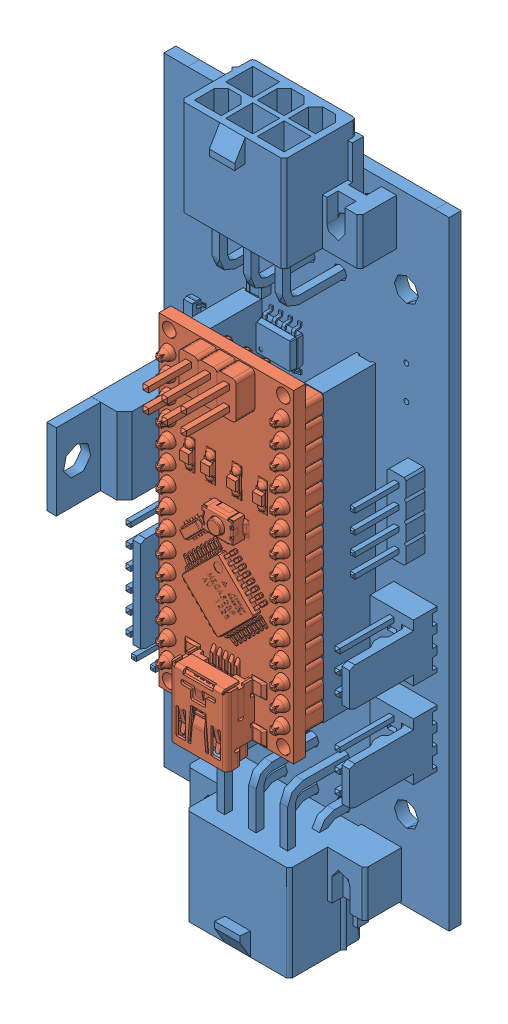
SolidWorks assembly DDI_AMPCD_Controller, configuration Default. Lengths in mm.
Overall size (38.1 94.5 29.35).
2 component instances, 2 part files, 6 mates.
Components (placement in the parent):
- ddi_ampcd_controller-1: ddi_ampcd_controller [Default] at origin size (38.1 94.5 28.52)
- arduino_nano-1: arduino_nano [Default] at (8.6868 59.4868 11.15) x (0 -1 0) z (-1 0 0) size (45 18.6 18)
Mates (geometry in assembly coordinates):
- Coincident1: coincident aligned: plane of ddi_ampcd_controller-1 through (0 0 0) normal (0 0 1)
- Coincident2: coincident aligned: plane of ddi_ampcd_controller-1 through (0 0 0) normal (0 1 0)
- Coincident3: coincident aligned: plane of ddi_ampcd_controller-1 through (0 0 0) normal (1 0 0)
- Width1: width: plane of ddi_ampcd_controller-1 through (7.4676 60.7568 1.65) normal (-1 0 0); plane of arduino_nano-1 through (25.146 22.733 1.65) normal (1 0 0); plane of ddi_ampcd_controller-1 through (25.3068 63.3068 38.4994) normal (1 0 0); plane of arduino_nano-1 through (7.3068 63.3068 38.4994) normal (-1 0 0)
- Width2: width: plane of ddi_ampcd_controller-1 through (7.4676 22.6568 1.65) normal (0 -1 0); plane of arduino_nano-1 through (10.0076 60.7568 1.65) normal (0 1 0); plane of ddi_ampcd_controller-1 through (9.4568 60.7568 34.3994) normal (0 1 0); plane of arduino_nano-1 through (7.9168 22.6568 34.3994) normal (0 -1 0)
- Coincident4: coincident anti-aligned: plane of ddi_ampcd_controller-1 through (10.0076 22.6568 8.65) normal (0 0 1); plane of arduino_nano-1 through (7.9168 58.7168 34.3994) normal (0 0 -1)
